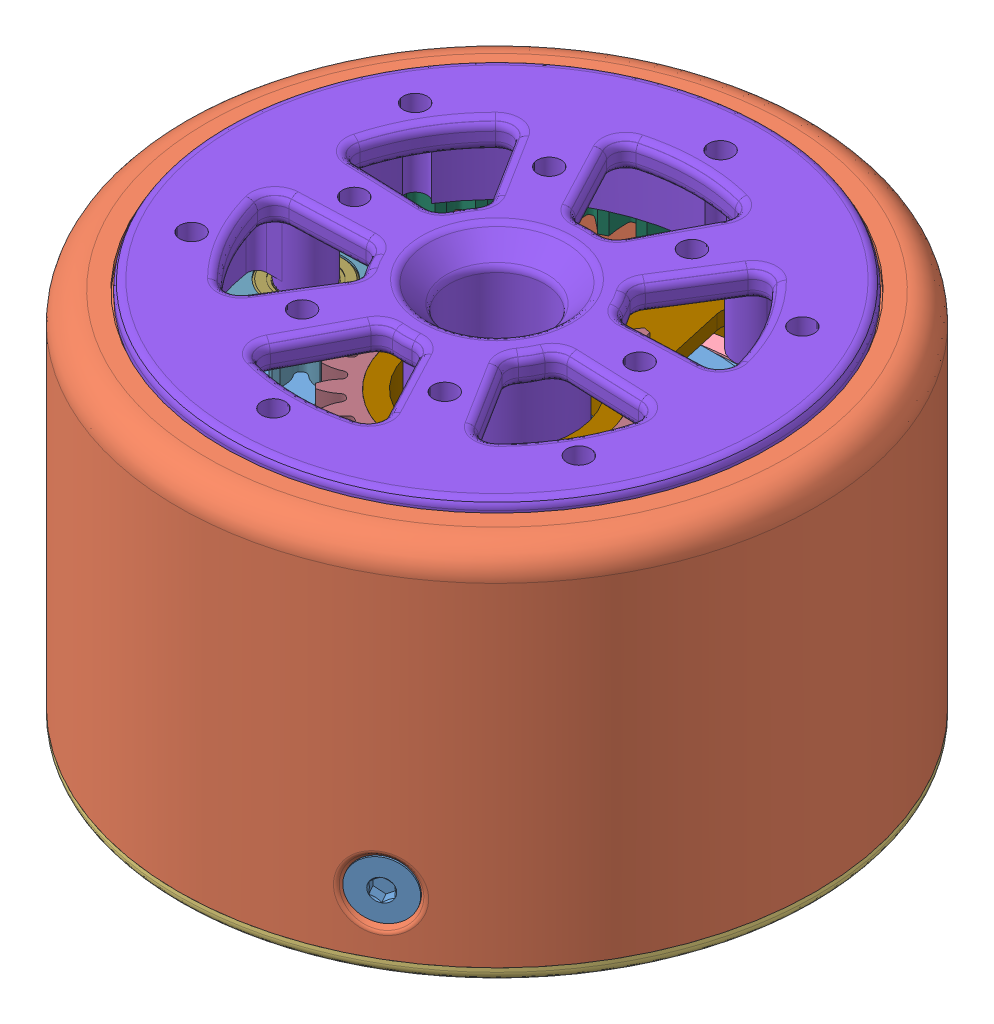
SolidWorks assembly ECG S assembly, configuration Default. Lengths in mm.
Overall size (67.08 41.65 67.03).
38 component instances, 19 part files, 38 mates.
Components (placement in the parent):
- Motor core S-1: Motor core S [Default] at origin size (51.8 14 51.8)
- Housing top-1: Housing top [Default] at origin size (67.06 38 67)
- Housing base-1: Housing base [Default] at origin size (67 19.41 67)
- Rotor magnet ring-1: Rotor magnet ring [Default] at (0 -10.75 0) size (60.8 10 60.8)
- M07900 slipring-1: M07900 slipring [Default] at (0 -8.2071 0) x (0.678989 0 -0.734148) z (0.734148 0 0.678989) size (7.9 13.8 7.9)
- PCB S-1: PCB S [Default] at (0 -13.4071 0) size (45 1.2 45)
- Magnetinc position ring-1: Magnetinc position ring [Default] at (0 -9.7071 0) x (0.334216 0 -0.942496) z (0.942496 0 0.334216) size (13 2.5 13)
- External rotor-1: External rotor [Default] at origin size (57 34.21 57)
- Internal rotor-1: Internal rotor [Default] at origin size (60.8 11 60.8)
- 6701 - 12x18x4 mm-3: 6701 - 12x18x4 mm [7804K116] at (0 8 0) x (0.913218 0 -0.407471) z (0 -1 0) size (18 18 4)
- 92000A076_18-8 SS METRIC PAN HEAD PHIL MACHINE SCREW-1: 92000A076_18-8 SS METRIC PAN HEAD PHIL MACHINE SCREW [92000A076] at (15.5 -10.4071 -15.5) x (0.994566 0 -0.104111) z (0 -1 0) size (6 6 8.6)
- 92000A076_18-8 SS METRIC PAN HEAD PHIL MACHINE SCREW-2: 92000A076_18-8 SS METRIC PAN HEAD PHIL MACHINE SCREW [92000A076] at (-15.5 -10.4071 -15.5) x (-0.284085 0 0.958799) z (0 -1 0) size (6 6 8.6)
- 92000A076_18-8 SS METRIC PAN HEAD PHIL MACHINE SCREW-3: 92000A076_18-8 SS METRIC PAN HEAD PHIL MACHINE SCREW [92000A076] at (-15.5 -10.4071 15.5) x (-0.074214 0 0.997242) z (0 -1 0) size (6 6 8.6)
- 92000A076_18-8 SS METRIC PAN HEAD PHIL MACHINE SCREW-4: 92000A076_18-8 SS METRIC PAN HEAD PHIL MACHINE SCREW [92000A076] at (15.5 -10.4071 15.5) x (0.991116 0 -0.133) z (0 -1 0) size (6 6 8.6)
- 7804K126_STAINLESS STEEL BALL BEARING-1: 7804K126_STAINLESS STEEL BALL BEARING [7804K126] at (-20.1 13 0) x (0.982591 0 0.185782) z (0 -1 0) size (8 8 4)
- Sun gear M1 Z25 bore 20-1: Sun gear M1 Z25 bore 20 [GearTrax] at (0 13 0) x (1 0 0) z (0 -1 0) size (27 27 4)
- Planet gear M1 Z15 bore 8-1: Planet gear M1 Z15 bore 8 [GearTrax] at (-20.1 13 0) x (1 0 0.000084) z (0 -1 0) size (17.2 17.2 4)
- Ring gear M1 Z55-1: Ring gear M1 Z55 [GearTrax] at (0 13 0) x (0.998367 0 -0.057121) z (0 -1 0) size (63 63 4)
- M1408-0120-2: M1408-0120 [Default] at (0 4.95 0) x (0.997046 0 0.076812) z (-0.076812 0 0.997046) size (15.2 1 15.18)
- Positioning magnet-1: Positioning magnet [Default] at (-12 6 0) x (0.68805 0 -0.725663) z (0.725663 0 0.68805) size (4 3 4)
- Positioning magnet-2: Positioning magnet [Default] at (-10.8116 6 5.2066) x (0.305058 0 -0.952334) z (0.952334 0 0.305058) size (4 3 4)
- Positioning magnet-3: Positioning magnet [Default] at (-7.4819 6 9.382) x (-0.138354 0 -0.990383) z (0.990383 0 -0.138354) size (4 3 4)
- Positioning magnet-4: Positioning magnet [Default] at (-2.6703 6 11.6991) x (-0.554364 0 -0.832275) z (0.832275 0 -0.554364) size (4 3 4)
- Positioning magnet-5: Positioning magnet [Default] at (2.6703 6 11.6991) x (-0.860575 0 -0.509324) z (0.509324 0 -0.860575) size (4 3 4)
- Positioning magnet-6: Positioning magnet [Default] at (7.4819 6 9.382) x (-0.996339 0 -0.085496) z (0.085496 0 -0.996339) size (4 3 4)
- Positioning magnet-7: Positioning magnet [Default] at (10.8116 6 5.2066) x (-0.934765 0 0.355266) z (-0.355266 0 -0.934765) size (4 3 4)
- Positioning magnet-8: Positioning magnet [Default] at (12 6 0) x (-0.68805 0 0.725663) z (-0.725663 0 -0.68805) size (4 3 4)
- Positioning magnet-9: Positioning magnet [Default] at (10.8116 6 -5.2066) x (-0.305058 0 0.952334) z (-0.952334 0 -0.305058) size (4 3 4)
- Positioning magnet-10: Positioning magnet [Default] at (7.4819 6 -9.382) x (0.138354 0 0.990383) z (-0.990383 0 0.138354) size (4 3 4)
- Positioning magnet-11: Positioning magnet [Default] at (2.6703 6 -11.6991) x (0.554364 0 0.832275) z (-0.832275 0 0.554364) size (4 3 4)
- Positioning magnet-12: Positioning magnet [Default] at (-2.6703 6 -11.6991) x (0.860575 0 0.509324) z (-0.509324 0 0.860575) size (4 3 4)
- Positioning magnet-13: Positioning magnet [Default] at (-7.4819 6 -9.382) x (0.996339 0 0.085496) z (-0.085496 0 0.996339) size (4 3 4)
- Positioning magnet-14: Positioning magnet [Default] at (-10.8116 6 -5.2066) x (0.934765 0 -0.355266) z (0.355266 0 0.934765) size (4 3 4)
- 6710 bearing 62x50x6 mm-1: 6710 bearing 62x50x6 mm [Default] at (0 16 0) x (0.996402 0 -0.084754) z (0.084754 0 0.996402) size (62 6 62)
- 6701 - 12x18x4 mm-4: 6701 - 12x18x4 mm [7804K116] at (0 -5.2071 0) x (0.933615 0 -0.358277) z (0 -1 0) size (18 18 4)
- M3x4 18-8 SS FLAT-HEAD SOCKET CAP SCREW-1: M3x4 18-8 SS FLAT-HEAD SOCKET CAP SCREW [92125A127] at (16.55 -8 -28.6654) x (-0.866025 0 -0.5) z (0.5 0 -0.866025) size (6 6 4.27)
- M3x4 18-8 SS FLAT-HEAD SOCKET CAP SCREW-2: M3x4 18-8 SS FLAT-HEAD SOCKET CAP SCREW [92125A127] at (-33.1 -8 0) x (0 0 1) z (-1 0 0) size (6 6 4.27)
- M3x4 18-8 SS FLAT-HEAD SOCKET CAP SCREW-3: M3x4 18-8 SS FLAT-HEAD SOCKET CAP SCREW [92125A127] at (16.55 -8 28.6654) x (0.866025 0 -0.5) z (0.5 0 0.866025) size (6 6 4.27)
Mates (geometry in assembly coordinates):
- Coincident2: coincident: line of M07900 slipring-1 through (69.0457 0 -8.2071) axis (0 0 1); line of assembly
- Parallel1: parallel: plane of PCB S-1 through (0 -13.4071 0) normal (0 0 1); plane of assembly through (0 0 0) normal (0 0 1)
- Concentric1: concentric: cylinder of PCB S-1 through (0 -12.2071 0) axis (0 -1 0) radius 3.5; line of assembly
- Concentric2: concentric: cylinder of Magnetinc position ring-1 through (0 -9.7071 0) axis (0 1 0) radius 4.15; line of assembly
- Width1: width: plane of Rotor magnet ring-1 through (-28.6579 4 5.0532) normal (0 1 0); plane of Rotor magnet ring-1 through (-24.8973 -4 15.0644) normal (0 -1 0); plane of Motor core S-1 through (-25.9 4 0) normal (0 1 0); plane of Motor core S-1 through (-25.9 -4 0) normal (0 -1 0)
- Concentric6: concentric: cylinder of PCB S-1 through (15.5 -12.2071 -15.5) axis (0 -1 0) radius 1.75; cylinder of 92000A076_18-8 SS METRIC PAN HEAD PHIL MACHINE SCREW-1 through (15.5 -10.4071 -15.5) axis (0 1 0) radius 3
- Coincident5: coincident: plane of PCB S-1 through (-11.5 -13.4071 11.5) normal (0 -1 0); plane of 92000A076_18-8 SS METRIC PAN HEAD PHIL MACHINE SCREW-1 through (15.5 -13.4071 -15.5) normal (0 1 0)
- Concentric7: concentric: cylinder of PCB S-1 through (-15.5 -12.2071 15.5) axis (0 -1 0) radius 1.75; cylinder of 92000A076_18-8 SS METRIC PAN HEAD PHIL MACHINE SCREW-3 through (-15.5 -10.4071 15.5) axis (0 1 0) radius 3
- Concentric8: concentric: cylinder of PCB S-1 through (15.5 -12.2071 15.5) axis (0 -1 0) radius 1.75; cylinder of 92000A076_18-8 SS METRIC PAN HEAD PHIL MACHINE SCREW-4 through (15.5 -10.4071 15.5) axis (0 1 0) radius 3
- Concentric9: concentric: cylinder of PCB S-1 through (-15.5 -12.2071 -15.5) axis (0 -1 0) radius 1.75; cylinder of 92000A076_18-8 SS METRIC PAN HEAD PHIL MACHINE SCREW-2 through (-15.5 -10.4071 -15.5) axis (0 1 0) radius 3
- Coincident6: coincident: plane of PCB S-1 through (-11.5 -13.4071 11.5) normal (0 -1 0); plane of 92000A076_18-8 SS METRIC PAN HEAD PHIL MACHINE SCREW-2 through (-15.5 -13.4071 -15.5) normal (0 1 0)
- Coincident7: coincident: plane of PCB S-1 through (-11.5 -13.4071 11.5) normal (0 -1 0); plane of 92000A076_18-8 SS METRIC PAN HEAD PHIL MACHINE SCREW-4 through (15.5 -13.4071 15.5) normal (0 1 0)
- Coincident8: coincident: plane of PCB S-1 through (-11.5 -13.4071 11.5) normal (0 -1 0); plane of 92000A076_18-8 SS METRIC PAN HEAD PHIL MACHINE SCREW-3 through (-15.5 -13.4071 15.5) normal (0 1 0)
- Concentric15: concentric: cylinder of External rotor-1 through (-20.098 18.273 0) axis (0 1 0) radius 1.48; cylinder of 7804K126_STAINLESS STEEL BALL BEARING-1 through (-20.098 9.65 0) axis (0 -1 0) radius 1.5
- Concentric19: concentric: cylinder of 6701 - 12x18x4 mm-3 through (0 6 0) axis (0 -1 0) radius 6; line of assembly
- Concentric21: concentric: cylinder of Sun gear M1 Z25 bore 20-1 through (0 13 0) axis (0 -1 0) radius 10; line of assembly
- Coincident17: coincident: plane of Internal rotor-1 through (-10 11 0) normal (0 1 0); plane of Sun gear M1 Z25 bore 20-1 through (0 11 0) normal (0 -1 0)
- Concentric22: concentric: cylinder of 7804K126_STAINLESS STEEL BALL BEARING-1 through (-20.1 11 0) axis (0 -1 0) radius 4; cylinder of Planet gear M1 Z15 bore 8-1 through (-20.1 13 0) axis (0 -1 0) radius 4
- Coincident18: coincident: plane of Sun gear M1 Z25 bore 20-1 through (0 15 13.5) normal (0 1 0); plane of Planet gear M1 Z15 bore 8-1 through (-20.1007 15 8.6) normal (0 1 0)
- Coincident19: coincident: plane of Planet gear M1 Z15 bore 8-1 through (-20.1007 15 8.6) normal (0 1 0); plane of Ring gear M1 Z55-1 through (1.7993 15 31.4486) normal (0 1 0)
- Concentric24: concentric: line of assembly; cylinder of Ring gear M1 Z55-1 through (0 13 0) axis (0 -1 0) radius 31.5
- Coincident20: coincident: plane of 7804K126_STAINLESS STEEL BALL BEARING-1 through (-20.806 11 3.7338) normal (0 -1 0); plane of Planet gear M1 Z15 bore 8-1 through (-20.1 11 0) normal (0 -1 0)
- Concentric25: concentric: cylinder of External rotor-1 through (-20.098 18.273 0) axis (0 1 0) radius 1.5; cylinder of 7804K126_STAINLESS STEEL BALL BEARING-1 through (-20.098 11 0) axis (0 -1 0) radius 1.5
- Coincident24: coincident: plane of Magnetinc position ring-1 through (-2.1724 -7.2071 6.1262) normal (0 1 0); plane of External rotor-1 through (-4.1 -7.2071 0) normal (0 -1 0)
- Coincident25: coincident: plane of M07900 slipring-1 through (-1.0185 -6.2071 1.1012) normal (0 -1 0); plane of External rotor-1 through (-4 -6.2071 0) normal (0 1 0)
- Coincident29: coincident: plane of Internal rotor-1 through (-11 10 0) normal (0 1 0); plane of 6701 - 12x18x4 mm-3 through (3.5857 10 8.0363) normal (0 1 0)
- Coincident31: coincident: line of M1408-0120-2 through (69.0457 0 4.95) axis (0 0 1); line of assembly
- Width3: width: plane of External rotor-1 through (-6.9577 4.9 0) normal (0 1 0); plane of External rotor-1 through (-6.9577 6 0) normal (0 -1 0); plane of M1408-0120-2 through (0 4.95 0) normal (0 -1 0); plane of M1408-0120-2 through (0 5.95 0) normal (0 1 0)
- Coincident32: coincident: plane of Internal rotor-1 through (0 0 0) normal (0 0 1); line of Positioning magnet-1 through (2.0534 -12 6) axis (0 0 1)
- Distance2: distance = 12 mm: line of Positioning magnet-1 through (2.0534 -12 6) axis (0 0 1); plane of Internal rotor-1 through (0 0 0) normal (1 0 0)
- Coincident33: coincident: line of 6710 bearing 62x50x6 mm-1 through (69.0457 0 16) axis (0 0 1); line of assembly
- Distance4: distance = 1 mm: plane of Ring gear M1 Z55-1 through (1.7993 15 31.4486) normal (0 1 0); plane of 6710 bearing 62x50x6 mm-1 through (-28.5782 16 2.4309) normal (0 -1 0)
- Coincident34: coincident: line of 6701 - 12x18x4 mm-4 through (0 -3.2071 0) axis (0 1 0); line of assembly
- Coincident36: coincident: plane of External rotor-1 through (-4.1 -7.2071 0) normal (0 -1 0); plane of 6701 - 12x18x4 mm-4 through (2.5613 -7.2071 6.6743) normal (0 -1 0)
- Concentric26: concentric: cylinder of External rotor-1 through (-20.1 18.273 0) axis (0 1 0) radius 1.5; cylinder of 7804K126_STAINLESS STEEL BALL BEARING-1 through (-20.1 11 0) axis (0 -1 0) radius 1.5
- Coincident38: coincident: cone of Housing top-1 through (15.75 -8 -27.2798) axis (-0.5 0 0.866025); cone of M3x4 18-8 SS FLAT-HEAD SOCKET CAP SCREW-1 through (15.7 -8 -27.1932) axis (-0.5 0 0.866025)
- Coincident40: coincident: cone of Housing top-1 through (-31.5 -8 0) axis (1 0 0); cone of M3x4 18-8 SS FLAT-HEAD SOCKET CAP SCREW-2 through (-31.4 -8 0) axis (1 0 0)
- Coincident41: coincident: cone of Housing top-1 through (15.75 -8 27.2798) axis (-0.5 0 -0.866025); cone of M3x4 18-8 SS FLAT-HEAD SOCKET CAP SCREW-3 through (15.7 -8 27.1932) axis (-0.5 0 -0.866025)
